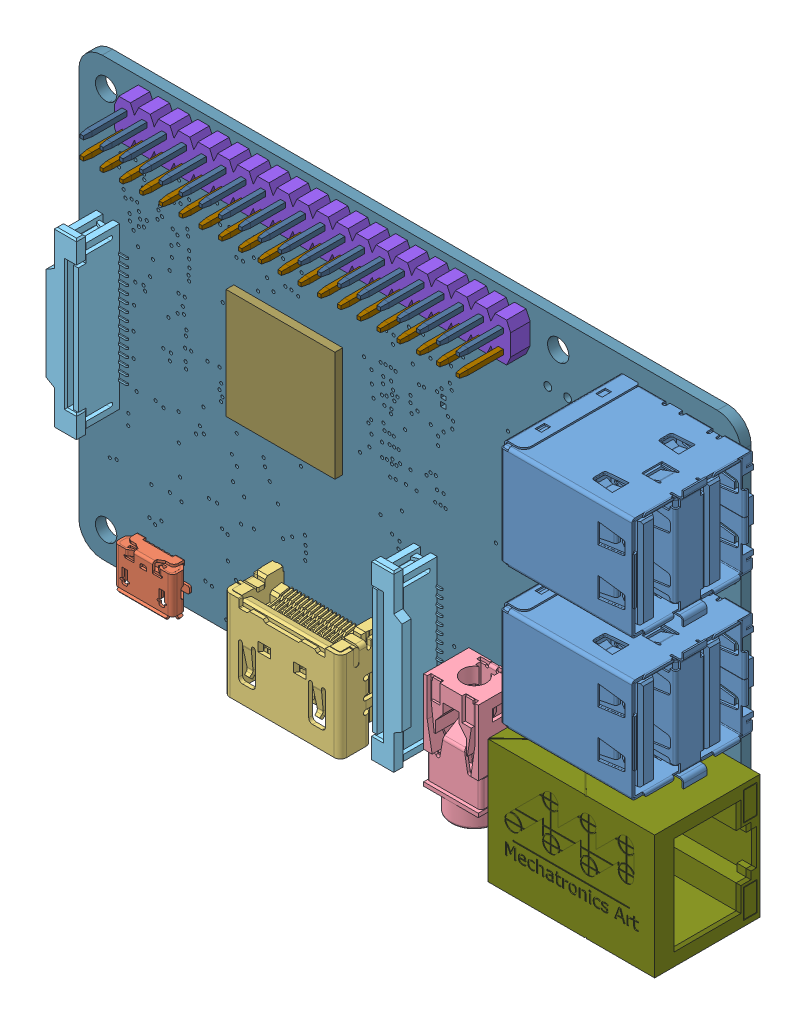
SolidWorks assembly Raspberry pi 3 cad model, configuration Default. Lengths in mm.
Overall size (89.64 57.31 18.59).
58 component instances, 16 part files, 0 mates.
Components (placement in the parent):
- raspberrypi_3_stripped.step-1: raspberrypi_3_stripped.step [Default] at origin size (89.64 57.31 18.59)
  - RPi3_ModelB v1.step-1: RPi3_ModelB v1.step [Default] at (-6 -61 0) x (1 0 0) z (0 -1 0) size (86.09 18.24 56.14)
    - MOLEX_672983090.step-1: MOLEX_672983090.step [Default] at (30.19 0.8 -64.5) x (0 0 -1) z (1 0 0) size (15.47 17.24 17.92)
    - MOLEX_672983090.step-2: MOLEX_672983090.step [Default] at (30.19 0.8 -82.5) x (0 0 -1) z (1 0 0) size (15.47 17.24 17.92)
    - molex_0473460001.step-1: molex_0473460001.step [Default] at (-31.9 0.8 -37.765) size (7.98 2.76 5.43)
    - molex_0471510001.step-1: molex_0471510001.step [Default] at (-10.5 0.65 -34.125) size (15.04 7.63 12.15)
    - PJ-322.step-1: PJ-322.step [Default] at (11.1 0.8 -42.85) size (7.23 7.55 15)
    - te_1-1734248-5.step-1: te_1-1734248-5.step [Default] at (-38.7109 0.8 -63.5) x (0 0 1) z (-1 0 0) size (22.4 5.68 5.07)
    - te_1-1734248-5.step-2: te_1-1734248-5.step [Default] at (2.058 0.82 -46.9107) x (0 0 -1) z (1 0 0) size (22.4 5.68 5.07)
    - MOLEX_1040310811.step-1: MOLEX_1040310811.step [Default] at (-35.065 -0.3 -63.58) x (0 0 -1) z (-1 0 0) size (11.95 1.45 11.4)
    - raspberry_pi_3(RJ45).step-1: raspberry_pi_3(RJ45).step [Default] at (44.6723 16.4551 -37.9773) x (0 0 -1) z (1 0 0) size (9.5 2.68 12.61)
  - Raspberry Pi 3157.step-1: Raspberry Pi 3157.step [Default] at origin size (50.8 5 2.5)
  - Raspberry Pi 3242.step-1: Raspberry Pi 3242.step [Default] at (0.3 0 0) size (0.64 0.64 5.5)
  - Raspberry Pi 3266.step-1: Raspberry Pi 3266.step [Default] at (0.3 -0.1777 0) size (0.64 0.64 5.5)
  - raspberry_pi_3(bar_180_2x20).step-1: raspberry_pi_3(bar_180_2x20).step [Default] at (-40.3908 28.1775 3.5) x (0 1 0) z (-1 0 0) size (3.19 3.1 48.91)
  - Raspberry Pi 312.step-1: Raspberry Pi 312.step [Default] at origin size (13.97 14.11 1)
  - Raspberry Pi 3180.step-1: Raspberry Pi 3180.step [Default] at origin size (0.5 0.3 0.3)
  - Raspberry Pi 31.step-1: Raspberry Pi 31.step [Default] at origin size (84.92 56 1.33)
  - raspberry_pi_B+_(microsd2).step-1: raspberry_pi_B+_(microsd2).step [Default] at (-43.2065 2.73 -0.97) x (1 0 0) z (0 1 0) size (15 0.97 11)
  - Raspberry Pi 3242.step-2: Raspberry Pi 3242.step [Default] at (2.84 0 0) size (0.64 0.64 5.5)
  - Raspberry Pi 3242.step-3: Raspberry Pi 3242.step [Default] at (5.38 0 0) size (0.64 0.64 5.5)
  - Raspberry Pi 3242.step-4: Raspberry Pi 3242.step [Default] at (7.92 0 0) size (0.64 0.64 5.5)
  - Raspberry Pi 3242.step-5: Raspberry Pi 3242.step [Default] at (10.46 0 0) size (0.64 0.64 5.5)
  - Raspberry Pi 3242.step-6: Raspberry Pi 3242.step [Default] at (13 0 0) size (0.64 0.64 5.5)
  - Raspberry Pi 3242.step-7: Raspberry Pi 3242.step [Default] at (15.54 0 0) size (0.64 0.64 5.5)
  - Raspberry Pi 3242.step-8: Raspberry Pi 3242.step [Default] at (18.08 0 0) size (0.64 0.64 5.5)
  - Raspberry Pi 3242.step-9: Raspberry Pi 3242.step [Default] at (20.62 0 0) size (0.64 0.64 5.5)
  - Raspberry Pi 3242.step-10: Raspberry Pi 3242.step [Default] at (23.16 0 0) size (0.64 0.64 5.5)
  - Raspberry Pi 3242.step-11: Raspberry Pi 3242.step [Default] at (25.7 0 0) size (0.64 0.64 5.5)
  - Raspberry Pi 3242.step-12: Raspberry Pi 3242.step [Default] at (28.24 0 0) size (0.64 0.64 5.5)
  - Raspberry Pi 3242.step-13: Raspberry Pi 3242.step [Default] at (30.78 0 0) size (0.64 0.64 5.5)
  - Raspberry Pi 3242.step-14: Raspberry Pi 3242.step [Default] at (33.32 0 0) size (0.64 0.64 5.5)
  - Raspberry Pi 3242.step-15: Raspberry Pi 3242.step [Default] at (35.86 0 0) size (0.64 0.64 5.5)
  - Raspberry Pi 3242.step-16: Raspberry Pi 3242.step [Default] at (38.4 0 0) size (0.64 0.64 5.5)
  - Raspberry Pi 3242.step-17: Raspberry Pi 3242.step [Default] at (40.94 0 0) size (0.64 0.64 5.5)
  - Raspberry Pi 3242.step-18: Raspberry Pi 3242.step [Default] at (43.48 0 0) size (0.64 0.64 5.5)
  - Raspberry Pi 3242.step-19: Raspberry Pi 3242.step [Default] at (46.02 0 0) size (0.64 0.64 5.5)
  - Raspberry Pi 3242.step-20: Raspberry Pi 3242.step [Default] at (48.56 0 0) size (0.64 0.64 5.5)
  - Raspberry Pi 3266.step-2: Raspberry Pi 3266.step [Default] at (2.84 -0.1777 0) size (0.64 0.64 5.5)
  - Raspberry Pi 3266.step-3: Raspberry Pi 3266.step [Default] at (5.38 -0.1777 0) size (0.64 0.64 5.5)
  - Raspberry Pi 3266.step-4: Raspberry Pi 3266.step [Default] at (7.92 -0.1777 0) size (0.64 0.64 5.5)
  - Raspberry Pi 3266.step-5: Raspberry Pi 3266.step [Default] at (10.46 -0.1777 0) size (0.64 0.64 5.5)
  - Raspberry Pi 3266.step-6: Raspberry Pi 3266.step [Default] at (13 -0.1777 0) size (0.64 0.64 5.5)
  - Raspberry Pi 3266.step-7: Raspberry Pi 3266.step [Default] at (15.54 -0.1777 0) size (0.64 0.64 5.5)
  - Raspberry Pi 3266.step-8: Raspberry Pi 3266.step [Default] at (18.08 -0.1777 0) size (0.64 0.64 5.5)
  - Raspberry Pi 3266.step-9: Raspberry Pi 3266.step [Default] at (20.62 -0.1777 0) size (0.64 0.64 5.5)
  - Raspberry Pi 3266.step-10: Raspberry Pi 3266.step [Default] at (23.16 -0.1777 0) size (0.64 0.64 5.5)
  - Raspberry Pi 3266.step-11: Raspberry Pi 3266.step [Default] at (25.7 -0.1777 0) size (0.64 0.64 5.5)
  - Raspberry Pi 3266.step-12: Raspberry Pi 3266.step [Default] at (28.24 -0.1777 0) size (0.64 0.64 5.5)
  - Raspberry Pi 3266.step-13: Raspberry Pi 3266.step [Default] at (30.78 -0.1777 0) size (0.64 0.64 5.5)
  - Raspberry Pi 3266.step-14: Raspberry Pi 3266.step [Default] at (33.32 -0.1777 0) size (0.64 0.64 5.5)
  - Raspberry Pi 3266.step-15: Raspberry Pi 3266.step [Default] at (35.86 -0.1777 0) size (0.64 0.64 5.5)
  - Raspberry Pi 3266.step-16: Raspberry Pi 3266.step [Default] at (38.4 -0.1777 0) size (0.64 0.64 5.5)
  - Raspberry Pi 3266.step-17: Raspberry Pi 3266.step [Default] at (40.94 -0.1777 0) size (0.64 0.64 5.5)
  - Raspberry Pi 3266.step-18: Raspberry Pi 3266.step [Default] at (43.48 -0.1777 0) size (0.64 0.64 5.5)
  - Raspberry Pi 3266.step-19: Raspberry Pi 3266.step [Default] at (46.02 -0.1777 0) size (0.64 0.64 5.5)
  - Raspberry Pi 3266.step-20: Raspberry Pi 3266.step [Default] at (48.56 -0.1777 0) size (0.64 0.64 5.5)
  - raspberry_pi_B_(RJ45).step-1: raspberry_pi_B_(RJ45).step [Default] at (38.93 -23.19 14.5) x (0 1 0) z (1 0 0) size (15.88 16.5 21.4)
